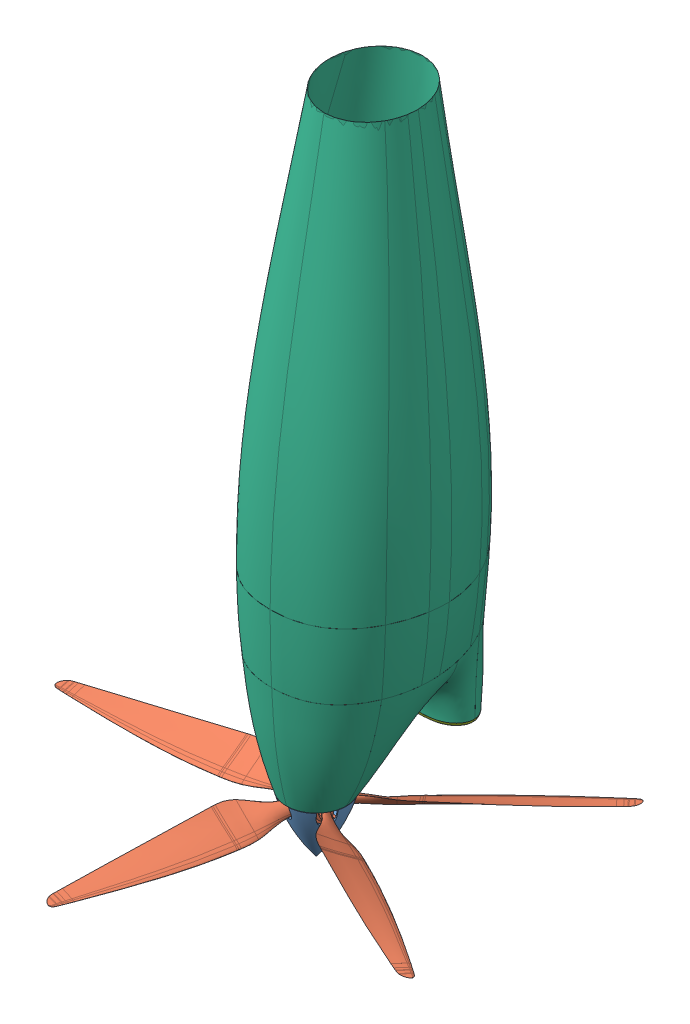
SolidWorks assembly turboprop engine, configuration 默认. Lengths in mm.
Overall size (11179.45 14556.69 11179.45).
7 component instances, 7 part files, 0 mates.
Components (placement in the parent):
- Part1-1: Part1 [默认] x (0.908506 0 -0.417872) z (0.417872 0 0.908506) size (1376.63 1323.22 1333.87)
- Part2-1: Part2 [默认] at (0 -119.3252 0) x (0.908045 0 -0.418873) z (0.418873 0 0.908045) size (9813.97 2487.64 9397.7)
- Part3-1: Part3 [默认] at origin size (2974.12 8746.18 3362.22)
- Part4-1: Part4 [默认] at origin size (2960.61 743.54 2960.61)
- Part5-1: Part5 [默认] at origin size (3105.35 7858.68 3105.35)
- Part6-1: Part6 [默认] at origin size (4416.85 14556.69 4314.79)
- Part6.5-1: Part6.5 [默认] at origin size (2360.92 70.68 1113.07)
